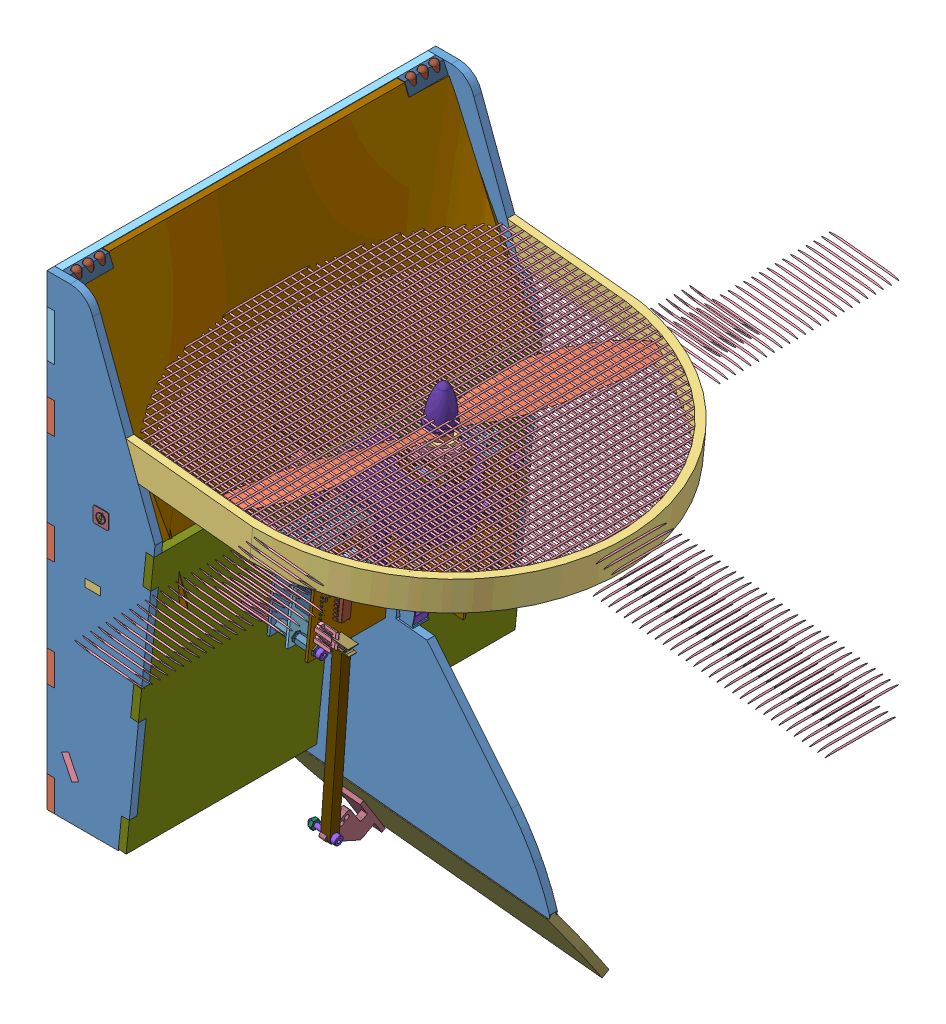
SolidWorks assembly AssTotaleSimu6, configuration Défaut. Lengths in mm. (continued)
Components (placement in the parent): (continued)
- AssStructSimu-1: AssStructSimu [Défaut] at (-125.7658 -1.8483 624.6548) x (1 0 0) z (0 0 -1) size (253.25 324.59 251.6) (continued)
  - AssCarte-1: AssCarte [Défaut] at (38.0121 147.1029 290.772) x (-0.101852 0.9948 0) z (0.9948 0.101852 0) size (66.52 130.57 98.72) (continued)
    - carte_onduleur_v3-1: carte_onduleur_v3 [Défaut] at (-131.8199 12.0892 20.7912) size (66.52 130.57 82.34) (continued)
      - U_DSPIC-1: U_DSPIC [Défaut] at (1.863 -2.61 0.803) size (7.92 35.56 7.75)
        - Open CASCADE STEP translator 6.8 1.17.1-1: Open CASCADE STEP translator 6.8 1.17.1 [Défaut] at origin size (7.92 35.56 7.75)
          - Body_1_4-1: Body_1_4 [Défaut] at (0 -0.2 4) x (1 0 0) z (0 -1 0) size (7.92 7.75 35.56)
      - C_DEC_DSPIC-1: C_DEC_DSPIC [Défaut] at (7.7 -8.8 -0.803) x (0 1 0) z (0 0 -1) size (2.34 1.04 0.5)
        - Open CASCADE STEP translator 6.8 1.6.1-1: Open CASCADE STEP translator 6.8 1.6.1 [Défaut] at origin size (2.34 1.04 0.5)
          - Body_1-1: Body_1 [Défaut] at origin size (2.29 1.04 0.43)
          - Pin_1-1: Pin_1 [Défaut] at (0.3048 0 0) x (-1 0 0) z (0 0 1) size (0.51 1.02 0.5)
          - Pin_2-1: Pin_2 [Défaut] at origin size (0.51 1.02 0.5)
      - IN-1: IN [Défaut] at (24.3 -5.3 0.803) x (0 1 0) z (0 0 1) size (10.21 15.56 26.9)
        - Open CASCADE STEP translator 6.8 1.19.1-1: Open CASCADE STEP translator 6.8 1.19.1 [Défaut] at origin size (10.21 15.56 26.9)
          - Body_1_3-1: Body_1_3 [Défaut] at (-13.5 1.8 3) x (0 1 0) z (1 0 0) size (15.56 26.9 10.21)
            - Imported-1: Imported [Défaut] at (2.0451 -4.5908 20.9802) size (8.6 15.9 10.16)
            - Imported-2: Imported [Défaut] at (-1.6683 9.1092 15.9802) x (0 0 1) z (-1 0 0) size (10.1 18.2 15.1)
              - Imported_2-1: Imported_2 [Défaut] at origin size (10.1 18.2 15.1)
              - Imported_3-1: Imported_3 [Défaut] at origin size (3.43 12.4 4.99)
              - Imported_4-1: Imported_4 [Défaut] at origin size (3.43 12.4 4.99)
              - Imported_5-1: Imported_5 [Défaut] at origin size (3.9 4.9 7)
              - Imported_6-1: Imported_6 [Défaut] at origin size (3.9 4.9 7)
              - Imported_7-1: Imported_7 [Défaut] at origin size (3.8 3.8 6.92)
              - Imported_8-1: Imported_8 [Défaut] at origin size (3.8 3.8 6.92)
              - Imported_9-1: Imported_9 [Défaut] at origin size (9 2.4 14.2)
      - CARTE_CMD-1: CARTE_CMD [Défaut] at (25 57.2 0.803) size (60.1 130 26.71)
        - Open CASCADE STEP translator 6.8 1.20.1-1: Open CASCADE STEP translator 6.8 1.20.1 [Défaut] at origin size (60.1 130 26.71)
          - Body_1_4-1: Body_1_4 [Défaut] at (-55 5 12) size (60.1 130 26.71)
            - 1_2-1: 1_2 [Défaut] at origin size (60.1 130 1.61)
            - 4-1: 4 [Défaut] at (23.6 -124.9 0.803) x (0 1 0) z (0 0 1) size (5 15.24 14.3)
              - =_[0_1_1_4]_2-1: =_[0_1_1_4]_2 [Défaut] at origin size (5 15.24 14.3)
                - 5-1: 5 [Défaut] at (0 -6.5 -13) x (0 1 0) z (0 0 -1) size (15.24 5 14.3)
            - 7-1: 7 [Défaut] at (23.6 -5 0.803) x (0 1 0) z (0 0 1) size (5 15.24 14.3)
              - =_[0_1_1_7]-1: =_[0_1_1_7] [Défaut] at origin size (5 15.24 14.3)
                - 5-1: 5 [Défaut] at (0 -6.5 -13) x (0 1 0) z (0 0 -1) size (15.24 5 14.3)
            - 10_2-1: 10_2 [Défaut] at (18.4 -115.6 0.803) size (25.4 7.92 7.75)
              - =_[0_1_1_9]-1: =_[0_1_1_9] [Défaut] at origin size (25.4 7.92 7.75)
                - 8-1: 8 [Défaut] at (11.2 4 0) x (0 1 0) z (1 0 0) size (7.92 7.75 25.4)
            - 13_2-1: 13_2 [Défaut] at (55.4 -114.7 0.803) x (-1 0 0) z (0 0 1) size (5 7.62 14.3)
              - =_[0_1_1_12]-1: =_[0_1_1_12] [Défaut] at origin size (5 7.62 14.3)
                - 11-1: 11 [Défaut] at (0 -2.5 11) x (0 -1 0) z (0 0 1) size (7.62 5 14.3)
            - 25-1: 25 [Défaut] at (56.9 -12.8 0.803) x (-1 0 0) z (0 0 1) size (16.02 47.26 11.05)
              - =_[0_1_1_15]_2-1: =_[0_1_1_15]_2 [Défaut] at origin size (16.02 47.26 11.05)
                - 23-1: 23 [Défaut] at (-36.5 21 4) x (0 -1 0) z (1 0 0) size (47.26 11.05 16.02)
                  - 14-1: 14 [Défaut] at (-7.4961 -1.5352 42.5833) size (42.58 6.55 16.01)
                  - 22-1: 22 [Défaut] at (19.3039 2.3748 37.905) x (-1 0 0) z (0 0 -1) size (10.36 6.14 15.24)
                    - 21-1: 21 [Défaut] at origin size (10.36 6.14 7.62)
                      - 19_2-1: 19_2 [Défaut] at origin size (10.36 6.14 2.54)
                        - 15-1: 15 [Défaut] at origin size (8.4 2.54 2.54)
                        - 16-1: 16 [Défaut] at (-0.0461 1.2682 1.27) x (0 0 -1) z (0.999998 -0.002105 0) size (1.95 5.07 7.58)
                      - 19_2-2: 19_2 [Défaut] at (0 0 -2.54) size (10.36 6.14 2.54)
                        - 15-1: 15 [Défaut] at origin size (8.4 2.54 2.54)
                        - 16-1: 16 [Défaut] at (-0.0461 1.2682 1.27) x (0 0 -1) z (0.999998 -0.002105 0) size (1.95 5.07 7.58)
                      - 19_2-3: 19_2 [Défaut] at (0 0 -5.08) size (10.36 6.14 2.54)
                        - 15-1: 15 [Défaut] at origin size (8.4 2.54 2.54)
                        - 16-1: 16 [Défaut] at (-0.0461 1.2682 1.27) x (0 0 -1) z (0.999998 -0.002105 0) size (1.95 5.07 7.58)
                    - 21-2: 21 [Défaut] at (0 0 -7.62) size (10.36 6.14 7.62)
                      - 19_2-1: 19_2 [Défaut] at origin size (10.36 6.14 2.54)
                        - 15-1: 15 [Défaut] at origin size (8.4 2.54 2.54)
                        - 16-1: 16 [Défaut] at (-0.0461 1.2682 1.27) x (0 0 -1) z (0.999998 -0.002105 0) size (1.95 5.07 7.58)
                      - 19_2-2: 19_2 [Défaut] at (0 0 -2.54) size (10.36 6.14 2.54)
                        - 15-1: 15 [Défaut] at origin size (8.4 2.54 2.54)
                        - 16-1: 16 [Défaut] at (-0.0461 1.2682 1.27) x (0 0 -1) z (0.999998 -0.002105 0) size (1.95 5.07 7.58)
                      - 19_2-3: 19_2 [Défaut] at (0 0 -5.08) size (10.36 6.14 2.54)
                        - 15-1: 15 [Défaut] at origin size (8.4 2.54 2.54)
                        - 16-1: 16 [Défaut] at (-0.0461 1.2682 1.27) x (0 0 -1) z (0.999998 -0.002105 0) size (1.95 5.07 7.58)
            - 31-1: 31 [Défaut] at (12.9 -104.5 0.803) size (6.76 3.64 4.37)
              - =_[0_1_1_24]-1: =_[0_1_1_24] [Défaut] at origin size (6.76 3.64 4.37)
                - 29-1: 29 [Défaut] at (-0.3 -2 0) size (6.76 3.64 4.37)
                  - =_[0_1_1_3]_3-1: =_[0_1_1_3]_3 [Défaut] at origin size (6 3.64 4.37)
                  - =_[0_1_1_4]_3-1: =_[0_1_1_4]_3 [Défaut] at origin size (0.38 1 0.67)
                  - =_[0_1_1_5]_3-1: =_[0_1_1_5]_3 [Défaut] at origin size (0.38 1 0.67)
            - 36-1: 36 [Défaut] at (28.6 -12.2 0.803) x (0 -1 0) z (0 0 1) size (2.34 1.04 0.5)
              - =_[0_1_1_30]-1: =_[0_1_1_30] [Défaut] at origin size (2.34 1.04 0.5)
                - 32_2-1: 32_2 [Défaut] at origin size (2.29 1.04 0.43)
                - 33_2-1: 33_2 [Défaut] at (0.3048 0 0) x (-1 0 0) z (0 0 1) size (0.51 1.02 0.5)
                - 34-1: 34 [Défaut] at origin size (0.51 1.02 0.5)
            - 38-1: 38 [Défaut] at (23.7 -12.2 0.803) x (0 -1 0) z (0 0 1) size (2.34 1.04 0.5)
              - =_[0_1_1_30]-1: =_[0_1_1_30] [Défaut] at origin size (2.34 1.04 0.5)
                - 32_2-1: 32_2 [Défaut] at origin size (2.29 1.04 0.43)
                - 33_2-1: 33_2 [Défaut] at (0.3048 0 0) x (-1 0 0) z (0 0 1) size (0.51 1.02 0.5)
                - 34-1: 34 [Défaut] at origin size (0.51 1.02 0.5)
            - 40_2-1: 40_2 [Défaut] at (26.2 -12.2 0.803) x (0 -1 0) z (0 0 1) size (2.34 1.04 0.5)
              - =_[0_1_1_30]-1: =_[0_1_1_30] [Défaut] at origin size (2.34 1.04 0.5)
                - 32_2-1: 32_2 [Défaut] at origin size (2.29 1.04 0.43)
                - 33_2-1: 33_2 [Défaut] at (0.3048 0 0) x (-1 0 0) z (0 0 1) size (0.51 1.02 0.5)
                - 34-1: 34 [Défaut] at origin size (0.51 1.02 0.5)
            - 42_2-1: 42_2 [Défaut] at (24.4 -119.2 0.803) size (2.34 1.04 0.5)
              - =_[0_1_1_30]-1: =_[0_1_1_30] [Défaut] at origin size (2.34 1.04 0.5)
                - 32_2-1: 32_2 [Défaut] at origin size (2.29 1.04 0.43)
                - 33_2-1: 33_2 [Défaut] at (0.3048 0 0) x (-1 0 0) z (0 0 1) size (0.51 1.02 0.5)
                - 34-1: 34 [Défaut] at origin size (0.51 1.02 0.5)
            - 45-1: 45 [Défaut] at (46.4 -125 0.803) size (5.08 5 14.3)
              - =_[0_1_1_38]-1: =_[0_1_1_38] [Défaut] at origin size (5.08 5 14.3)
                - 46-1: 46 [Défaut] at (1.2 0 11) size (5.08 5 14.3)
            - 48-1: 48 [Défaut] at (40.1 -125 0.803) size (5.08 5 14.3)
              - =_[0_1_1_41]-1: =_[0_1_1_41] [Défaut] at origin size (5.08 5 14.3)
                - 46-1: 46 [Défaut] at (1.2 0 11) size (5.08 5 14.3)
            - 51-1: 51 [Défaut] at (6.4 -119.9 0.803) x (0 1 0) z (0 0 1) size (15.24 2.54 7.37)
              - =_[0_1_1_43]-1: =_[0_1_1_43] [Défaut] at origin size (15.24 2.54 7.37)
                - 49_2-1: 49_2 [Défaut] at (6.5 0 0) x (1 0 0) z (0 -1 0) size (15.24 7.37 2.54)
            - 57_2-1: 57_2 [Défaut] at (50.8796 -121.1 -0.803) x (-1 0 0) z (0 0 -1) size (2.54 1.98 0.64)
              - =_[0_1_1_46]-1: =_[0_1_1_46] [Défaut] at origin size (2.54 1.98 0.64)
                - 52-1: 52 [Défaut] at origin size (2.54 1.14 0.58)
                - 53-1: 53 [Défaut] x (0 -1 0) z (0 0 1) size (0.43 0.51 0.38)
                - 54-1: 54 [Défaut] at (1.8796 1.8796 0) x (0 -1 0) z (0 0 1) size (0.43 0.51 0.38)
                - 55-1: 55 [Défaut] at (-0.9652 -2.8448 0) x (0 1 0) z (0 0 1) size (0.41 0.51 0.38)
            - 59_2-1: 59_2 [Défaut] at (43.6398 -120.995 -0.803) x (-1 0 0) z (0 0 -1) size (2.54 1.98 0.64)
              - =_[0_1_1_46]-1: =_[0_1_1_46] [Défaut] at origin size (2.54 1.98 0.64)
                - 52-1: 52 [Défaut] at origin size (2.54 1.14 0.58)
                - 53-1: 53 [Défaut] x (0 -1 0) z (0 0 1) size (0.43 0.51 0.38)
                - 54-1: 54 [Défaut] at (1.8796 1.8796 0) x (0 -1 0) z (0 0 1) size (0.43 0.51 0.38)
                - 55-1: 55 [Défaut] at (-0.9652 -2.8448 0) x (0 1 0) z (0 0 1) size (0.41 0.51 0.38)
            - 61_2-1: 61_2 [Défaut] at (47.6 -119.9 -0.803) x (-1 0 0) z (0 0 -1) size (2.34 1.04 0.5)
              - =_[0_1_1_30]-1: =_[0_1_1_30] [Défaut] at origin size (2.34 1.04 0.5)
                - 32_2-1: 32_2 [Défaut] at origin size (2.29 1.04 0.43)
                - 33_2-1: 33_2 [Défaut] at (0.3048 0 0) x (-1 0 0) z (0 0 1) size (0.51 1.02 0.5)
                - 34-1: 34 [Défaut] at origin size (0.51 1.02 0.5)
            - 63-1: 63 [Défaut] at (40.4 -119.9 -0.803) x (-1 0 0) z (0 0 -1) size (2.34 1.04 0.5)
              - =_[0_1_1_30]-1: =_[0_1_1_30] [Défaut] at origin size (2.34 1.04 0.5)
                - 32_2-1: 32_2 [Défaut] at origin size (2.29 1.04 0.43)
                - 33_2-1: 33_2 [Défaut] at (0.3048 0 0) x (-1 0 0) z (0 0 1) size (0.51 1.02 0.5)
                - 34-1: 34 [Défaut] at origin size (0.51 1.02 0.5)
            - 68-1: 68 [Défaut] at (47.7 -21.8 -0.803) x (0 1 0) z (0 0 -1) size (2.34 1.04 0.5)
              - =_[0_1_1_55]-1: =_[0_1_1_55] [Défaut] at origin size (2.34 1.04 0.5)
                - 64-1: 64 [Défaut] at origin size (2.29 1.04 0.43)
                - 65-1: 65 [Défaut] at (0.3048 0 0) x (-1 0 0) z (0 0 1) size (0.51 1.02 0.5)
                - 66-1: 66 [Défaut] at origin size (0.51 1.02 0.5)
            - 70-1: 70 [Défaut] at (47.6 -121.7 -0.803) x (-1 0 0) z (0 0 -1) size (2.34 1.04 0.5)
              - =_[0_1_1_30]-1: =_[0_1_1_30] [Défaut] at origin size (2.34 1.04 0.5)
                - 32_2-1: 32_2 [Défaut] at origin size (2.29 1.04 0.43)
                - 33_2-1: 33_2 [Défaut] at (0.3048 0 0) x (-1 0 0) z (0 0 1) size (0.51 1.02 0.5)
                - 34-1: 34 [Défaut] at origin size (0.51 1.02 0.5)
            - 72_2-1: 72_2 [Défaut] at (40.4 -121.5 -0.803) x (-1 0 0) z (0 0 -1) size (2.34 1.04 0.5)
              - =_[0_1_1_30]-1: =_[0_1_1_30] [Défaut] at origin size (2.34 1.04 0.5)
                - 32_2-1: 32_2 [Défaut] at origin size (2.29 1.04 0.43)
                - 33_2-1: 33_2 [Défaut] at (0.3048 0 0) x (-1 0 0) z (0 0 1) size (0.51 1.02 0.5)
                - 34-1: 34 [Défaut] at origin size (0.51 1.02 0.5)
            - 74_2-1: 74_2 [Défaut] at (47.7 -18.3 -0.803) x (0 1 0) z (0 0 -1) size (2.34 1.04 0.5)
              - =_[0_1_1_55]-1: =_[0_1_1_55] [Défaut] at origin size (2.34 1.04 0.5)
                - 64-1: 64 [Défaut] at origin size (2.29 1.04 0.43)
                - 65-1: 65 [Défaut] at (0.3048 0 0) x (-1 0 0) z (0 0 1) size (0.51 1.02 0.5)
                - 66-1: 66 [Défaut] at origin size (0.51 1.02 0.5)
            - 76_2-1: 76_2 [Défaut] at (45.5 -118.3 -0.803) x (1 0 0) z (0 0 -1) size (2.34 1.04 0.5)
              - =_[0_1_1_30]-1: =_[0_1_1_30] [Défaut] at origin size (2.34 1.04 0.5)
                - 32_2-1: 32_2 [Défaut] at origin size (2.29 1.04 0.43)
                - 33_2-1: 33_2 [Défaut] at (0.3048 0 0) x (-1 0 0) z (0 0 1) size (0.51 1.02 0.5)
                - 34-1: 34 [Défaut] at origin size (0.51 1.02 0.5)
            - 78_2-1: 78_2 [Défaut] at (38.2 -118.3 -0.803) x (1 0 0) z (0 0 -1) size (2.34 1.04 0.5)
              - =_[0_1_1_30]-1: =_[0_1_1_30] [Défaut] at origin size (2.34 1.04 0.5)
                - 32_2-1: 32_2 [Défaut] at origin size (2.29 1.04 0.43)
                - 33_2-1: 33_2 [Défaut] at (0.3048 0 0) x (-1 0 0) z (0 0 1) size (0.51 1.02 0.5)
                - 34-1: 34 [Défaut] at origin size (0.51 1.02 0.5)
            - 80_2-1: 80_2 [Défaut] at (28.6 -10.7 0.803) x (0 1 0) z (0 0 1) size (2.34 1.04 0.5)
              - =_[0_1_1_55]-1: =_[0_1_1_55] [Défaut] at origin size (2.34 1.04 0.5)
                - 64-1: 64 [Défaut] at origin size (2.29 1.04 0.43)
                - 65-1: 65 [Défaut] at (0.3048 0 0) x (-1 0 0) z (0 0 1) size (0.51 1.02 0.5)
                - 66-1: 66 [Défaut] at origin size (0.51 1.02 0.5)
            - 82_2-1: 82_2 [Défaut] at (23.7 -10.7 0.803) x (0 1 0) z (0 0 1) size (2.34 1.04 0.5)
              - =_[0_1_1_55]-1: =_[0_1_1_55] [Défaut] at origin size (2.34 1.04 0.5)
                - 64-1: 64 [Défaut] at origin size (2.29 1.04 0.43)
                - 65-1: 65 [Défaut] at (0.3048 0 0) x (-1 0 0) z (0 0 1) size (0.51 1.02 0.5)
                - 66-1: 66 [Défaut] at origin size (0.51 1.02 0.5)
            - 84-1: 84 [Défaut] at (26.2 -10.7 0.803) x (0 1 0) z (0 0 1) size (2.34 1.04 0.5)
              - =_[0_1_1_55]-1: =_[0_1_1_55] [Défaut] at origin size (2.34 1.04 0.5)
                - 64-1: 64 [Défaut] at origin size (2.29 1.04 0.43)
                - 65-1: 65 [Défaut] at (0.3048 0 0) x (-1 0 0) z (0 0 1) size (0.51 1.02 0.5)
                - 66-1: 66 [Défaut] at origin size (0.51 1.02 0.5)
            - 86-1: 86 [Défaut] at (23.0336 -119.2 0.803) x (-1 0 0) z (0 0 1) size (2.34 1.04 0.5)
              - =_[0_1_1_55]-1: =_[0_1_1_55] [Défaut] at origin size (2.34 1.04 0.5)
                - 64-1: 64 [Défaut] at origin size (2.29 1.04 0.43)
                - 65-1: 65 [Défaut] at (0.3048 0 0) x (-1 0 0) z (0 0 1) size (0.51 1.02 0.5)
                - 66-1: 66 [Défaut] at origin size (0.51 1.02 0.5)
            - 88-1: 88 [Défaut] at (14.1 -114.2 0.803) x (0 -1 0) z (0 0 1) size (2.34 1.04 0.5)
              - =_[0_1_1_55]-1: =_[0_1_1_55] [Défaut] at origin size (2.34 1.04 0.5)
                - 64-1: 64 [Défaut] at origin size (2.29 1.04 0.43)
                - 65-1: 65 [Défaut] at (0.3048 0 0) x (-1 0 0) z (0 0 1) size (0.51 1.02 0.5)
                - 66-1: 66 [Défaut] at origin size (0.51 1.02 0.5)
            - 90-1: 90 [Défaut] at (43.6 -107.8 -0.803) x (1 0 0) z (0 0 -1) size (2.34 1.04 0.5)
              - =_[0_1_1_55]-1: =_[0_1_1_55] [Défaut] at origin size (2.34 1.04 0.5)
                - 64-1: 64 [Défaut] at origin size (2.29 1.04 0.43)
                - 65-1: 65 [Défaut] at (0.3048 0 0) x (-1 0 0) z (0 0 1) size (0.51 1.02 0.5)
                - 66-1: 66 [Défaut] at origin size (0.51 1.02 0.5)
            - 92-1: 92 [Défaut] at (43.6 -106 -0.803) x (1 0 0) z (0 0 -1) size (2.34 1.04 0.5)
              - =_[0_1_1_55]-1: =_[0_1_1_55] [Défaut] at origin size (2.34 1.04 0.5)
                - 64-1: 64 [Défaut] at origin size (2.29 1.04 0.43)
                - 65-1: 65 [Défaut] at (0.3048 0 0) x (-1 0 0) z (0 0 1) size (0.51 1.02 0.5)
                - 66-1: 66 [Défaut] at origin size (0.51 1.02 0.5)
            - 175-1: 175 [Défaut] at (10 -21.7 0.803) x (0 -1 0) z (0 0 1) size (15 25.4 12.78)
              - =_[0_1_1_72]-1: =_[0_1_1_72] [Défaut] at origin size (15 25.4 12.78)
                - 173-1: 173 [Défaut] at (-1.4 -1 12) x (-1 0 0) z (0 1 0) size (15 12.78 25.4)
                  - board_1-1: board_1 [Défaut] at (-7.5 -1.57 12.5) size (15 1.57 25)
                  - hole_plating_20-1: hole_plating_20 [Défaut] at (-1.5 0 23.93) size (1.5 0.01 1.5)
                  - hole_plating_20-2: hole_plating_20 [Défaut] at (-1.5 0 21.39) size (1.5 0.01 1.5)
                  - hole_plating_20-3: hole_plating_20 [Défaut] at (-1.5 0 8.69) size (1.5 0.01 1.5)
                  - hole_plating_20-4: hole_plating_20 [Défaut] at (-1.5 -1.58 13.77) size (1.5 0.01 1.5)
                  - hole_plating_20-5: hole_plating_20 [Défaut] at (-1.5 0 16.31) size (1.5 0.01 1.5)
                  - hole_plating_20-6: hole_plating_20 [Défaut] at (-1.5 0 18.85) size (1.5 0.01 1.5)
                  - hole_plating_20-7: hole_plating_20 [Défaut] at (-1.5 0 13.77) size (1.5 0.01 1.5)
                  - hole_plating_20-8: hole_plating_20 [Défaut] at (-1.5 -1.58 11.23) size (1.5 0.01 1.5)
                  - hole_plating_20-9: hole_plating_20 [Défaut] at (-1.5 -1.58 18.85) size (1.5 0.01 1.5)
                  - hole_plating_20-10: hole_plating_20 [Défaut] at (-1.5 -1.58 6.15) size (1.5 0.01 1.5)
                  - hole_plating_20-11: hole_plating_20 [Défaut] at (-1.5 0 1.07) size (1.5 0.01 1.5)
                  - hole_plating_20-12: hole_plating_20 [Défaut] at (-1.5 -1.58 3.61) size (1.5 0.01 1.5)
                  - hole_plating_20-13: hole_plating_20 [Défaut] at (-1.5 -1.58 1.07) size (1.5 0.01 1.5)
                  - hole_plating_20-14: hole_plating_20 [Défaut] at (-1.5 -1.58 8.69) size (1.5 0.01 1.5)
                  - hole_plating_20-15: hole_plating_20 [Défaut] at (-1.5 -1.58 16.31) size (1.5 0.01 1.5)
                  - hole_plating_20-16: hole_plating_20 [Défaut] at (-1.5 0 11.23) size (1.5 0.01 1.5)
                  - hole_plating_20-17: hole_plating_20 [Défaut] at (-1.5 0 3.61) size (1.5 0.01 1.5)
                  - hole_plating_20-18: hole_plating_20 [Défaut] at (-1.5 -1.58 21.39) size (1.5 0.01 1.5)
                  - hole_plating_20-19: hole_plating_20 [Défaut] at (-1.5 0 6.15) size (1.5 0.01 1.5)
                  - hole_plating_20-20: hole_plating_20 [Défaut] at (-1.5 -1.58 23.93) size (1.5 0.01 1.5)
                  - Pin_Header_1x10_TH_Pitch_2.54mm_1-1: Pin_Header_1x10_TH_Pitch_2.54mm_1 [Défaut] at (-1.5 -1.5786 23.93) x (0 0 -1) z (0 -1 0) size (25.4 2.54 12.7)
                    - 124-1: 124 [Défaut] at origin size (25.4 2.54 2.8)
                      - =_[0_1_1_77]-1: =_[0_1_1_77] [Défaut] at origin size (2.54 2.54 2.8)
                      - =_[0_1_1_79]-1: =_[0_1_1_79] [Défaut] at origin size (2.54 2.54 2.8)
                      - =_[0_1_1_80]-1: =_[0_1_1_80] [Défaut] at origin size (2.54 2.54 2.8)
                      - =_[0_1_1_81]-1: =_[0_1_1_81] [Défaut] at origin size (2.54 2.54 2.8)
                      - =_[0_1_1_82]-1: =_[0_1_1_82] [Défaut] at origin size (2.54 2.54 2.8)
                      - =_[0_1_1_83]-1: =_[0_1_1_83] [Défaut] at origin size (2.54 2.54 2.8)
                      - =_[0_1_1_84]-1: =_[0_1_1_84] [Défaut] at origin size (2.54 2.54 2.8)
                      - =_[0_1_1_85]-1: =_[0_1_1_85] [Défaut] at origin size (2.54 2.54 2.8)
                      - =_[0_1_1_86]-1: =_[0_1_1_86] [Défaut] at origin size (2.54 2.54 2.8)
                      - =_[0_1_1_87]-1: =_[0_1_1_87] [Défaut] at origin size (2.54 2.54 2.8)
                    - 135-1: 135 [Défaut] at origin size (23.49 0.63 12.7)
                      - =_[0_1_1_88]-1: =_[0_1_1_88] [Défaut] at origin size (0.63 0.63 12.7)
                      - =_[0_1_1_90]-1: =_[0_1_1_90] [Défaut] at origin size (0.63 0.63 12.7)
                      - =_[0_1_1_91]-1: =_[0_1_1_91] [Défaut] at origin size (0.63 0.63 12.7)
                      - =_[0_1_1_92]-1: =_[0_1_1_92] [Défaut] at origin size (0.63 0.63 12.7)
                      - =_[0_1_1_93]-1: =_[0_1_1_93] [Défaut] at origin size (0.63 0.63 12.7)
                      - =_[0_1_1_94]-1: =_[0_1_1_94] [Défaut] at origin size (0.63 0.63 12.7)
                      - =_[0_1_1_95]-1: =_[0_1_1_95] [Défaut] at origin size (0.63 0.63 12.7)
                      - =_[0_1_1_96]-1: =_[0_1_1_96] [Défaut] at origin size (0.63 0.63 12.7)
                      - =_[0_1_1_97]-1: =_[0_1_1_97] [Défaut] at origin size (0.63 0.63 12.7)
                      - =_[0_1_1_98]-1: =_[0_1_1_98] [Défaut] at origin size (0.63 0.63 12.7)
                  - MPU-9250_1-1: MPU-9250_1 [Défaut] at (-8 0.05 12.5) x (-1 0 0) z (0 1 0) size (3 3 1.05)
                  - tantalum_10uF_1-1: tantalum_10uF_1 [Défaut] at (-13.167 0.1 10.9372) x (0 0 1) z (0 1 0) size (3.4 1.6 1.71)
                  - SOT23_5_1-1: SOT23_5_1 [Défaut] at (-7.475 -0.0136 21) x (0 0 1) z (0 1 0) size (3 3.2 0.92)
                  - RESC-0603_5-1: RESC-0603_5 [Défaut] at (-6.85 0 7.45) x (1 0 0) z (0 1 0) size (1.7 0.9 0.55)
                    - 143-1: 143 [Défaut] at origin size (1.7 0.9 0.55)
                      - =_[0_1_1_103]-1: =_[0_1_1_103] [Défaut] at origin size (0.4 0.9 0.53)
                      - =_[0_1_1_105]-1: =_[0_1_1_105] [Défaut] at origin size (0.4 0.9 0.53)
                      - =_[0_1_1_106]-1: =_[0_1_1_106] [Défaut] at origin size (1.64 0.9 0.52)
                    - 152-1: 152 [Défaut] at origin
                      - =_[0_1_1_107]-1: =_[0_1_1_107] [Défaut] at origin
                      - =_[0_1_1_109]-1: =_[0_1_1_109] [Défaut] at origin
                      - =_[0_1_1_110]-1: =_[0_1_1_110] [Défaut] at origin
                      - =_[0_1_1_111]-1: =_[0_1_1_111] [Défaut] at origin
                      - =_[0_1_1_112]-1: =_[0_1_1_112] [Défaut] at origin
                      - =_[0_1_1_113]-1: =_[0_1_1_113] [Défaut] at origin
                      - =_[0_1_1_114]-1: =_[0_1_1_114] [Défaut] at origin
                      - =_[0_1_1_115]-1: =_[0_1_1_115] [Défaut] at origin
                  - RESC-0603_5-2: RESC-0603_5 [Défaut] at (-9.85 0 16.05) x (1 0 0) z (0 1 0) size (1.7 0.9 0.55)
                    - 143-1: 143 [Défaut] at origin size (1.7 0.9 0.55)
                      - =_[0_1_1_103]-1: =_[0_1_1_103] [Défaut] at origin size (0.4 0.9 0.53)
                      - =_[0_1_1_105]-1: =_[0_1_1_105] [Défaut] at origin size (0.4 0.9 0.53)
                      - =_[0_1_1_106]-1: =_[0_1_1_106] [Défaut] at origin size (1.64 0.9 0.52)
                    - 152-1: 152 [Défaut] at origin
                      - =_[0_1_1_107]-1: =_[0_1_1_107] [Défaut] at origin
                      - =_[0_1_1_109]-1: =_[0_1_1_109] [Défaut] at origin
                      - =_[0_1_1_110]-1: =_[0_1_1_110] [Défaut] at origin
                      - =_[0_1_1_111]-1: =_[0_1_1_111] [Défaut] at origin
                      - =_[0_1_1_112]-1: =_[0_1_1_112] [Défaut] at origin
                      - =_[0_1_1_113]-1: =_[0_1_1_113] [Défaut] at origin
                      - =_[0_1_1_114]-1: =_[0_1_1_114] [Défaut] at origin
                      - =_[0_1_1_115]-1: =_[0_1_1_115] [Défaut] at origin
                  - RESC-0603_5-3: RESC-0603_5 [Défaut] at (-6.85 0 17.55) x (1 0 0) z (0 1 0) size (1.7 0.9 0.55)
                    - 143-1: 143 [Défaut] at origin size (1.7 0.9 0.55)
                      - =_[0_1_1_103]-1: =_[0_1_1_103] [Défaut] at origin size (0.4 0.9 0.53)
                      - =_[0_1_1_105]-1: =_[0_1_1_105] [Défaut] at origin size (0.4 0.9 0.53)
                      - =_[0_1_1_106]-1: =_[0_1_1_106] [Défaut] at origin size (1.64 0.9 0.52)
                    - 152-1: 152 [Défaut] at origin
                      - =_[0_1_1_107]-1: =_[0_1_1_107] [Défaut] at origin
                      - =_[0_1_1_109]-1: =_[0_1_1_109] [Défaut] at origin
                      - =_[0_1_1_110]-1: =_[0_1_1_110] [Défaut] at origin
                      - =_[0_1_1_111]-1: =_[0_1_1_111] [Défaut] at origin
                      - =_[0_1_1_112]-1: =_[0_1_1_112] [Défaut] at origin
                      - =_[0_1_1_113]-1: =_[0_1_1_113] [Défaut] at origin
                      - =_[0_1_1_114]-1: =_[0_1_1_114] [Défaut] at origin
                      - =_[0_1_1_115]-1: =_[0_1_1_115] [Défaut] at origin
                  - RESC-0603_5-4: RESC-0603_5 [Défaut] at (-6.85 0 16.05) x (1 0 0) z (0 1 0) size (1.7 0.9 0.55)
                    - 143-1: 143 [Défaut] at origin size (1.7 0.9 0.55)
                      - =_[0_1_1_103]-1: =_[0_1_1_103] [Défaut] at origin size (0.4 0.9 0.53)
                      - =_[0_1_1_105]-1: =_[0_1_1_105] [Défaut] at origin size (0.4 0.9 0.53)
                      - =_[0_1_1_106]-1: =_[0_1_1_106] [Défaut] at origin size (1.64 0.9 0.52)
                    - 152-1: 152 [Défaut] at origin
                      - =_[0_1_1_107]-1: =_[0_1_1_107] [Défaut] at origin
                      - =_[0_1_1_109]-1: =_[0_1_1_109] [Défaut] at origin
                      - =_[0_1_1_110]-1: =_[0_1_1_110] [Défaut] at origin
                      - =_[0_1_1_111]-1: =_[0_1_1_111] [Défaut] at origin
                      - =_[0_1_1_112]-1: =_[0_1_1_112] [Défaut] at origin
                      - =_[0_1_1_113]-1: =_[0_1_1_113] [Défaut] at origin
                      - =_[0_1_1_114]-1: =_[0_1_1_114] [Défaut] at origin
                      - =_[0_1_1_115]-1: =_[0_1_1_115] [Défaut] at origin
                  - RESC-0603_5-5: RESC-0603_5 [Défaut] at (-6.85 0 5.95) x (1 0 0) z (0 1 0) size (1.7 0.9 0.55)
                    - 143-1: 143 [Défaut] at origin size (1.7 0.9 0.55)
                      - =_[0_1_1_103]-1: =_[0_1_1_103] [Défaut] at origin size (0.4 0.9 0.53)
                      - =_[0_1_1_105]-1: =_[0_1_1_105] [Défaut] at origin size (0.4 0.9 0.53)
                      - =_[0_1_1_106]-1: =_[0_1_1_106] [Défaut] at origin size (1.64 0.9 0.52)
                    - 152-1: 152 [Défaut] at origin
                      - =_[0_1_1_107]-1: =_[0_1_1_107] [Défaut] at origin
                      - =_[0_1_1_109]-1: =_[0_1_1_109] [Défaut] at origin
                      - =_[0_1_1_110]-1: =_[0_1_1_110] [Défaut] at origin
                      - =_[0_1_1_111]-1: =_[0_1_1_111] [Défaut] at origin
                      - =_[0_1_1_112]-1: =_[0_1_1_112] [Défaut] at origin
                      - =_[0_1_1_113]-1: =_[0_1_1_113] [Défaut] at origin
                      - =_[0_1_1_114]-1: =_[0_1_1_114] [Défaut] at origin
                      - =_[0_1_1_115]-1: =_[0_1_1_115] [Défaut] at origin
                  - CAPC-0603-T0.9-BN_5-1: CAPC-0603-T0.9-BN_5 [Défaut] at (-9.85 0 8.95) x (1 0 0) z (0 1 0) size (1.7 0.9 0.9)
                    - =_[0_1_1_117]-1: =_[0_1_1_117] [Défaut] at origin size (1.7 0.9 0.9)
                    - 167-1: 167 [Défaut] at origin
                      - =_[0_1_1_118]-1: =_[0_1_1_118] [Défaut] at origin
                      - =_[0_1_1_120]-1: =_[0_1_1_120] [Défaut] at origin
                      - =_[0_1_1_121]-1: =_[0_1_1_121] [Défaut] at origin
                      - =_[0_1_1_122]-1: =_[0_1_1_122] [Défaut] at origin
                      - =_[0_1_1_123]-1: =_[0_1_1_123] [Défaut] at origin
                      - =_[0_1_1_124]-1: =_[0_1_1_124] [Défaut] at origin
                      - =_[0_1_1_125]-1: =_[0_1_1_125] [Défaut] at origin
                      - =_[0_1_1_126]-1: =_[0_1_1_126] [Défaut] at origin
                  - CAPC-0603-T0.9-BN_5-2: CAPC-0603-T0.9-BN_5 [Défaut] at (-6.85 0 8.95) x (1 0 0) z (0 1 0) size (1.7 0.9 0.9)
                    - =_[0_1_1_117]-1: =_[0_1_1_117] [Défaut] at origin size (1.7 0.9 0.9)
                    - 167-1: 167 [Défaut] at origin
                      - =_[0_1_1_118]-1: =_[0_1_1_118] [Défaut] at origin
                      - =_[0_1_1_120]-1: =_[0_1_1_120] [Défaut] at origin
                      - =_[0_1_1_121]-1: =_[0_1_1_121] [Défaut] at origin
                      - =_[0_1_1_122]-1: =_[0_1_1_122] [Défaut] at origin
                      - =_[0_1_1_123]-1: =_[0_1_1_123] [Défaut] at origin
                      - =_[0_1_1_124]-1: =_[0_1_1_124] [Défaut] at origin
                      - =_[0_1_1_125]-1: =_[0_1_1_125] [Défaut] at origin
                      - =_[0_1_1_126]-1: =_[0_1_1_126] [Défaut] at origin
                  - CAPC-0603-T0.9-BN_5-3: CAPC-0603-T0.9-BN_5 [Défaut] at (-6.85 0 19.05) x (1 0 0) z (0 1 0) size (1.7 0.9 0.9)
                    - =_[0_1_1_117]-1: =_[0_1_1_117] [Défaut] at origin size (1.7 0.9 0.9)
                    - 167-1: 167 [Défaut] at origin
                      - =_[0_1_1_118]-1: =_[0_1_1_118] [Défaut] at origin
                      - =_[0_1_1_120]-1: =_[0_1_1_120] [Défaut] at origin
                      - =_[0_1_1_121]-1: =_[0_1_1_121] [Défaut] at origin
                      - =_[0_1_1_122]-1: =_[0_1_1_122] [Défaut] at origin
                      - =_[0_1_1_123]-1: =_[0_1_1_123] [Défaut] at origin
                      - =_[0_1_1_124]-1: =_[0_1_1_124] [Défaut] at origin
                      - =_[0_1_1_125]-1: =_[0_1_1_125] [Défaut] at origin
                      - =_[0_1_1_126]-1: =_[0_1_1_126] [Défaut] at origin
                  - CAPC-0603-T0.9-BN_5-4: CAPC-0603-T0.9-BN_5 [Défaut] at (-9.85 0 7.45) x (1 0 0) z (0 1 0) size (1.7 0.9 0.9)
                    - =_[0_1_1_117]-1: =_[0_1_1_117] [Défaut] at origin size (1.7 0.9 0.9)
                    - 167-1: 167 [Défaut] at origin
                      - =_[0_1_1_118]-1: =_[0_1_1_118] [Défaut] at origin
                      - =_[0_1_1_120]-1: =_[0_1_1_120] [Défaut] at origin
                      - =_[0_1_1_121]-1: =_[0_1_1_121] [Défaut] at origin
                      - =_[0_1_1_122]-1: =_[0_1_1_122] [Défaut] at origin
                      - =_[0_1_1_123]-1: =_[0_1_1_123] [Défaut] at origin
                      - =_[0_1_1_124]-1: =_[0_1_1_124] [Défaut] at origin
                      - =_[0_1_1_125]-1: =_[0_1_1_125] [Défaut] at origin
                      - =_[0_1_1_126]-1: =_[0_1_1_126] [Défaut] at origin
                  - CAPC-0603-T0.9-BN_5-5: CAPC-0603-T0.9-BN_5 [Défaut] at (-9.85 0 17.55) x (1 0 0) z (0 1 0) size (1.7 0.9 0.9)
                    - =_[0_1_1_117]-1: =_[0_1_1_117] [Défaut] at origin size (1.7 0.9 0.9)
                    - 167-1: 167 [Défaut] at origin
                      - =_[0_1_1_118]-1: =_[0_1_1_118] [Défaut] at origin
                      - =_[0_1_1_120]-1: =_[0_1_1_120] [Défaut] at origin
                      - =_[0_1_1_121]-1: =_[0_1_1_121] [Défaut] at origin
                      - =_[0_1_1_122]-1: =_[0_1_1_122] [Défaut] at origin
                      - =_[0_1_1_123]-1: =_[0_1_1_123] [Défaut] at origin
                      - =_[0_1_1_124]-1: =_[0_1_1_124] [Défaut] at origin
                      - =_[0_1_1_125]-1: =_[0_1_1_125] [Défaut] at origin
                      - =_[0_1_1_126]-1: =_[0_1_1_126] [Défaut] at origin
            - 177-1: 177 [Défaut] at (52.1 -16.5 -0.803) x (1 0 0) z (0 0 -1) size (2.34 1.04 0.5)
              - =_[0_1_1_30]-1: =_[0_1_1_30] [Défaut] at origin size (2.34 1.04 0.5)
                - 32_2-1: 32_2 [Défaut] at origin size (2.29 1.04 0.43)
                - 33_2-1: 33_2 [Défaut] at (0.3048 0 0) x (-1 0 0) z (0 0 1) size (0.51 1.02 0.5)
                - 34-1: 34 [Défaut] at origin size (0.51 1.02 0.5)
            - 179-1: 179 [Défaut] at (22.5336 -121.5 -0.803) x (-1 0 0) z (0 0 -1) size (2.34 1.04 0.5)
              - =_[0_1_1_30]-1: =_[0_1_1_30] [Défaut] at origin size (2.34 1.04 0.5)
                - 32_2-1: 32_2 [Défaut] at origin size (2.29 1.04 0.43)
                - 33_2-1: 33_2 [Défaut] at (0.3048 0 0) x (-1 0 0) z (0 0 1) size (0.51 1.02 0.5)
                - 34-1: 34 [Défaut] at origin size (0.51 1.02 0.5)
            - 181-1: 181 [Défaut] at (48.6 -127 -0.803) x (-1 0 0) z (0 0 -1) size (2.34 1.04 0.5)
              - =_[0_1_1_30]-1: =_[0_1_1_30] [Défaut] at origin size (2.34 1.04 0.5)
                - 32_2-1: 32_2 [Défaut] at origin size (2.29 1.04 0.43)
                - 33_2-1: 33_2 [Défaut] at (0.3048 0 0) x (-1 0 0) z (0 0 1) size (0.51 1.02 0.5)
                - 34-1: 34 [Défaut] at origin size (0.51 1.02 0.5)
            - 183-1: 183 [Défaut] at (26.0189 -121.5 0.803) size (2.34 1.04 0.5)
              - =_[0_1_1_30]-1: =_[0_1_1_30] [Défaut] at origin size (2.34 1.04 0.5)
                - 32_2-1: 32_2 [Défaut] at origin size (2.29 1.04 0.43)
                - 33_2-1: 33_2 [Défaut] at (0.3048 0 0) x (-1 0 0) z (0 0 1) size (0.51 1.02 0.5)
                - 34-1: 34 [Défaut] at origin size (0.51 1.02 0.5)
            - 185-1: 185 [Défaut] at (30.3664 -19 -0.803) x (1 0 0) z (0 0 -1) size (2.34 1.04 0.5)
              - =_[0_1_1_30]-1: =_[0_1_1_30] [Défaut] at origin size (2.34 1.04 0.5)
                - 32_2-1: 32_2 [Défaut] at origin size (2.29 1.04 0.43)
                - 33_2-1: 33_2 [Défaut] at (0.3048 0 0) x (-1 0 0) z (0 0 1) size (0.51 1.02 0.5)
                - 34-1: 34 [Défaut] at origin size (0.51 1.02 0.5)
            - 187-1: 187 [Défaut] at (51.7 -114.3 -0.803) x (0 1 0) z (0 0 -1) size (2.34 1.04 0.5)
              - =_[0_1_1_30]-1: =_[0_1_1_30] [Défaut] at origin size (2.34 1.04 0.5)
                - 32_2-1: 32_2 [Défaut] at origin size (2.29 1.04 0.43)
                - 33_2-1: 33_2 [Défaut] at (0.3048 0 0) x (-1 0 0) z (0 0 1) size (0.51 1.02 0.5)
                - 34-1: 34 [Défaut] at origin size (0.51 1.02 0.5)
            - 189-1: 189 [Défaut] at (50 -114.3 -0.803) x (0 1 0) z (0 0 -1) size (2.34 1.04 0.5)
              - =_[0_1_1_30]-1: =_[0_1_1_30] [Défaut] at origin size (2.34 1.04 0.5)
                - 32_2-1: 32_2 [Défaut] at origin size (2.29 1.04 0.43)
                - 33_2-1: 33_2 [Défaut] at (0.3048 0 0) x (-1 0 0) z (0 0 1) size (0.51 1.02 0.5)
                - 34-1: 34 [Défaut] at origin size (0.51 1.02 0.5)
      - C2_1-1: C2_1 [Défaut] at (-20.6984 1.8 -0.803) x (1 0 0) z (0 0 -1) size (2.34 1.04 0.5)
        - Open CASCADE STEP translator 6.8 1.6.1-1: Open CASCADE STEP translator 6.8 1.6.1 [Défaut] at origin size (2.34 1.04 0.5)
          - Body_1-1: Body_1 [Défaut] at origin size (2.29 1.04 0.43)
          - Pin_1-1: Pin_1 [Défaut] at (0.3048 0 0) x (-1 0 0) z (0 0 1) size (0.51 1.02 0.5)
          - Pin_2-1: Pin_2 [Défaut] at origin size (0.51 1.02 0.5)
      - C2_2-1: C2_2 [Défaut] at (-24.2 1.8 -0.803) x (1 0 0) z (0 0 -1) size (2.34 1.04 0.5)
        - Open CASCADE STEP translator 6.8 1.6.1-1: Open CASCADE STEP translator 6.8 1.6.1 [Défaut] at origin size (2.34 1.04 0.5)
          - Body_1-1: Body_1 [Défaut] at origin size (2.29 1.04 0.43)
          - Pin_1-1: Pin_1 [Défaut] at (0.3048 0 0) x (-1 0 0) z (0 0 1) size (0.51 1.02 0.5)
          - Pin_2-1: Pin_2 [Défaut] at origin size (0.51 1.02 0.5)
      - C3_1-1: C3_1 [Défaut] at (-20.9176 -12.8 -0.803) x (1 0 0) z (0 0 -1) size (2.34 1.04 0.5)
        - Open CASCADE STEP translator 6.8 1.6.1-1: Open CASCADE STEP translator 6.8 1.6.1 [Défaut] at origin size (2.34 1.04 0.5)
          - Body_1-1: Body_1 [Défaut] at origin size (2.29 1.04 0.43)
          - Pin_1-1: Pin_1 [Défaut] at (0.3048 0 0) x (-1 0 0) z (0 0 1) size (0.51 1.02 0.5)
          - Pin_2-1: Pin_2 [Défaut] at origin size (0.51 1.02 0.5)
      - C3_2-1: C3_2 [Défaut] at (-24.4 -12.8 -0.803) x (1 0 0) z (0 0 -1) size (2.34 1.04 0.5)
        - Open CASCADE STEP translator 6.8 1.6.1-1: Open CASCADE STEP translator 6.8 1.6.1 [Défaut] at origin size (2.34 1.04 0.5)
          - Body_1-1: Body_1 [Défaut] at origin size (2.29 1.04 0.43)
          - Pin_1-1: Pin_1 [Défaut] at (0.3048 0 0) x (-1 0 0) z (0 0 1) size (0.51 1.02 0.5)
          - Pin_2-1: Pin_2 [Défaut] at origin size (0.51 1.02 0.5)
      - D_CUR-1: D_CUR [Défaut] at (-12.4432 3.85 -0.803) x (0 -1 0) z (0 0 -1) size (2.7 5.2 1.11)
        - Open CASCADE STEP translator 6.8 1.25.1-1: Open CASCADE STEP translator 6.8 1.25.1 [Défaut] at origin size (2.7 5.2 1.11)
          - Body_1_5-1: Body_1_5 [Défaut] at (1.2 -4 0) x (0 1 0) z (0 0 1) size (5.2 2.7 1.11)
            - =_[0_1_1_3]_4-1: =_[0_1_1_3]_4 [Défaut] at origin size (0.39 0.64 0.01)
            - =_[0_1_1_4]_4-1: =_[0_1_1_4]_4 [Défaut] at origin size (0.6 1.9 0.2)
            - =_[0_1_1_5]_4-1: =_[0_1_1_5]_4 [Défaut] at origin size (0.21 0.08 0.01)
            - =_[0_1_1_6]_2-1: =_[0_1_1_6]_2 [Défaut] at origin size (0.6 1.9 0.2)
            - =_[0_1_1_7]_2-1: =_[0_1_1_7]_2 [Défaut] at origin size (0.46 0.68 0.01)
            - =_[0_1_1_8]_2-1: =_[0_1_1_8]_2 [Défaut] at origin size (0.38 0.66 0.01)
            - =_[0_1_1_9]-1: =_[0_1_1_9] [Défaut] at origin size (0.2 0.62 0.01)
            - =_[0_1_1_10]-1: =_[0_1_1_10] [Défaut] at origin size (4 2.7 1.1)
            - =_[0_1_1_11]-1: =_[0_1_1_11] [Défaut] at origin size (0.46 0.63 0.01)
            - =_[0_1_1_12]-1: =_[0_1_1_12] [Défaut] at origin size (0.56 0.68 0.01)
      - RC1_1-1: RC1_1 [Défaut] at (-20.7176 8.1 -0.803) x (1 0 0) z (0 0 -1) size (2.34 1.04 0.5)
        - Open CASCADE STEP translator 6.8 1.12.1-1: Open CASCADE STEP translator 6.8 1.12.1 [Défaut] at origin size (2.34 1.04 0.5)
          - Body_1_3-1: Body_1_3 [Défaut] at origin size (2.29 1.04 0.43)
          - Pin_1_2-1: Pin_1_2 [Défaut] at (0.3048 0 0) x (-1 0 0) z (0 0 1) size (0.51 1.02 0.5)
          - Pin_2_2-1: Pin_2_2 [Défaut] at origin size (0.51 1.02 0.5)
      - RC1_2-1: RC1_2 [Défaut] at (-22 8.1 -0.803) x (-1 0 0) z (0 0 -1) size (2.34 1.04 0.5)
        - Open CASCADE STEP translator 6.8 1.12.1-1: Open CASCADE STEP translator 6.8 1.12.1 [Défaut] at origin size (2.34 1.04 0.5)
          - Body_1_3-1: Body_1_3 [Défaut] at origin size (2.29 1.04 0.43)
          - Pin_1_2-1: Pin_1_2 [Défaut] at (0.3048 0 0) x (-1 0 0) z (0 0 1) size (0.51 1.02 0.5)
          - Pin_2_2-1: Pin_2_2 [Défaut] at origin size (0.51 1.02 0.5)
      - RC2_1-1: RC2_1 [Défaut] at (-20.716 0.243 -0.803) x (1 0 0) z (0 0 -1) size (2.34 1.04 0.5)
        - Open CASCADE STEP translator 6.8 1.12.1-1: Open CASCADE STEP translator 6.8 1.12.1 [Défaut] at origin size (2.34 1.04 0.5)
          - Body_1_3-1: Body_1_3 [Défaut] at origin size (2.29 1.04 0.43)
          - Pin_1_2-1: Pin_1_2 [Défaut] at (0.3048 0 0) x (-1 0 0) z (0 0 1) size (0.51 1.02 0.5)
          - Pin_2_2-1: Pin_2_2 [Défaut] at origin size (0.51 1.02 0.5)
      - RC2_2-1: RC2_2 [Défaut] at (-22 0.18 -0.803) x (-1 0 0) z (0 0 -1) size (2.34 1.04 0.5)
        - Open CASCADE STEP translator 6.8 1.12.1-1: Open CASCADE STEP translator 6.8 1.12.1 [Défaut] at origin size (2.34 1.04 0.5)
          - Body_1_3-1: Body_1_3 [Défaut] at origin size (2.29 1.04 0.43)
          - Pin_1_2-1: Pin_1_2 [Défaut] at (0.3048 0 0) x (-1 0 0) z (0 0 1) size (0.51 1.02 0.5)
